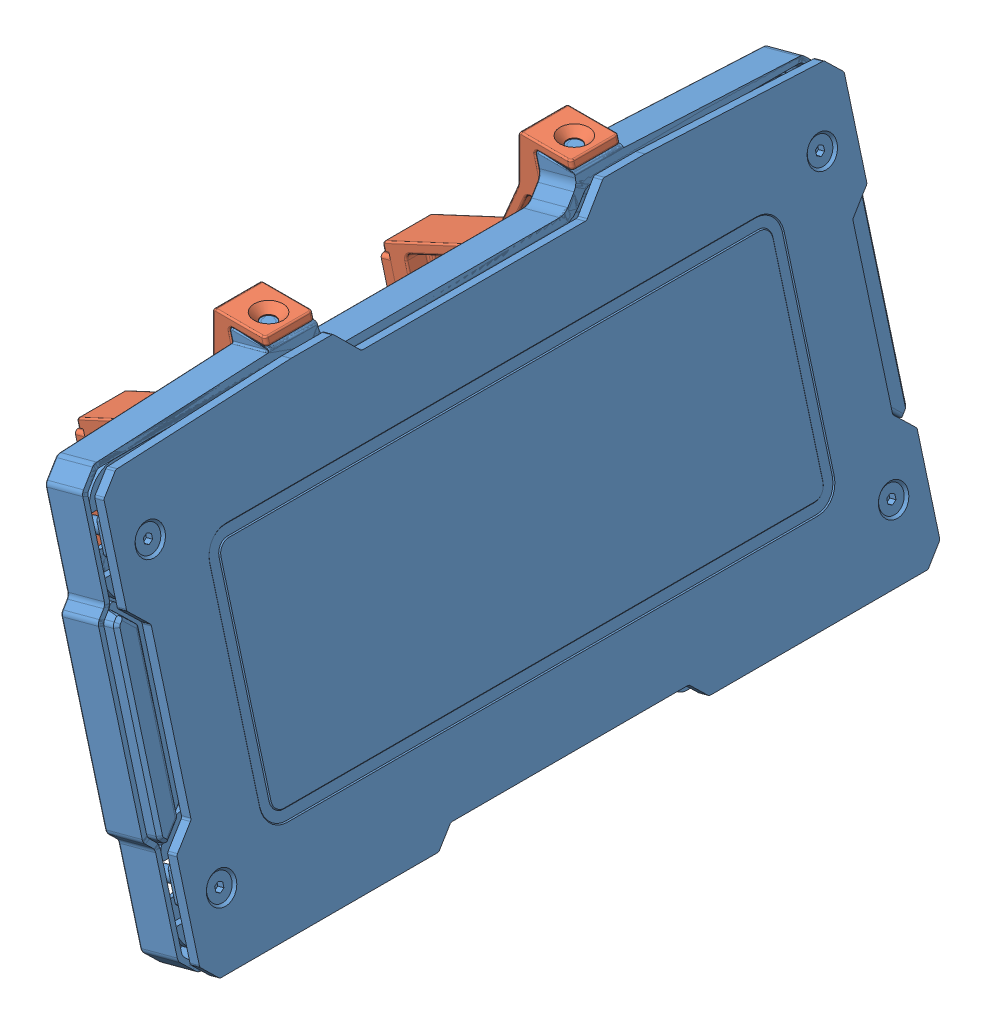
SolidWorks assembly 大装甲模块, configuration 默认. Lengths in mm.
Overall size (110.83 141.2 236.09).
4 component instances, 3 part files, 9 mates.
Components (placement in the parent):
- 复件 大装甲^大装甲模块-1: 复件 大装甲^大装甲模块 [默认] at (-90.092 0.6932 236.1184) size (53.57 127.71 236.09) (virtual)
- 复件 装甲支撑架^大装甲模块-2: 复件 装甲支撑架^大装甲模块 [默认] at (-37.0051 -26.5885 283.6184) x (0 0 1) z (-0.965926 -0.258819 0) size (15.02 127.12 71.15) (virtual)
- 复件 装甲支撑架^大装甲模块-3: 复件 装甲支撑架^大装甲模块 [默认] at (-37.0051 -26.5885 188.6184) x (0 0 1) z (-0.965926 -0.258819 0) size (15.02 127.12 71.15) (virtual)
- 复件 大装甲角度检测^大装甲模块-1: 复件 大装甲角度检测^大装甲模块 [Default] at (30.5522 13.5489 236.1184) x (0 0 -1) z (0.965926 0.258819 0) size (1086.89 983.89 300) (hidden, virtual)
Mates (geometry in assembly coordinates):
- 重合1: coincident anti-aligned: plane of 复件 大装甲^大装甲模块-1 through (-5.5852 75.0053 276.1184) normal (0 1 0); plane of 复件 装甲支撑架^大装甲模块-2 through (6.3204 75.0053 308.8036) normal (0 -1 0)
- 重合2: coincident anti-aligned: plane of 复件 大装甲^大装甲模块-1 through (12.1996 8.6313 236.1184) normal (-0.965926 -0.258819 0); plane of 复件 装甲支撑架^大装甲模块-2 through (-5.5852 75.0053 276.1184) normal (0.965926 0.258819 0)
- 同心1: concentric anti-aligned: circle of 复件 大装甲^大装甲模块-1; cylinder of 复件 装甲支撑架^大装甲模块-2 through (-0.6619 77.5053 283.6184) axis (0 1 0) radius 2.25
- 重合3: coincident anti-aligned: plane of 复件 大装甲^大装甲模块-1 through (12.1996 8.6313 236.1184) normal (-0.965926 -0.258819 0); plane of 复件 装甲支撑架^大装甲模块-3 through (-5.5852 75.0053 181.1184) normal (0.965926 0.258819 0)
- 重合4: coincident anti-aligned: plane of 复件 大装甲^大装甲模块-1 through (-5.5852 75.0053 196.1184) normal (0 1 0); plane of 复件 装甲支撑架^大装甲模块-3 through (6.3204 75.0053 213.8036) normal (0 -1 0)
- 同心2: concentric anti-aligned: circle of 复件 大装甲^大装甲模块-1; cylinder of 复件 装甲支撑架^大装甲模块-3 through (-0.6619 77.5053 188.6184) axis (0 1 0) radius 2.25
- 重合5: coincident anti-aligned: plane of 复件 大装甲^大装甲模块-1 through (30.5522 13.5489 236.1184) normal (0.965926 0.258819 0); plane of 复件 大装甲角度检测^大装甲模块-1 through (30.5522 13.5489 236.1184) normal (-0.965926 -0.258819 0)
- 宽度3: width aligned: plane of 复件 大装甲角度检测^大装甲模块-1 through (46.9872 -47.7874 121.1184) normal (-0.79124 -0.212012 -0.573576); plane of 复件 大装甲角度检测^大装甲模块-1 through (46.9872 -47.7874 351.1184) normal (-0.79124 -0.212012 0.573576); plane of 复件 大装甲^大装甲模块-1 through (30.5522 13.5489 345.1184) normal (0 0 1); plane of 复件 大装甲^大装甲模块-1 through (30.5522 13.5489 127.1184) normal (0 0 -1)
- 宽度4: width aligned: plane of 复件 大装甲角度检测^大装甲模块-1 through (46.9872 -47.7874 351.1184) normal (-0.642788 -0.766044 0); plane of 复件 大装甲角度检测^大装甲模块-1 through (14.1172 74.8852 351.1184) normal (-0.939693 0.34202 0); plane of 复件 大装甲^大装甲模块-1 through (6.0109 66.5015 176.1184) normal (-0.258819 0.965926 0); plane of 复件 大装甲^大装甲模块-1 through (35.7751 -44.58 176.1184) normal (0.258819 -0.965926 0)
